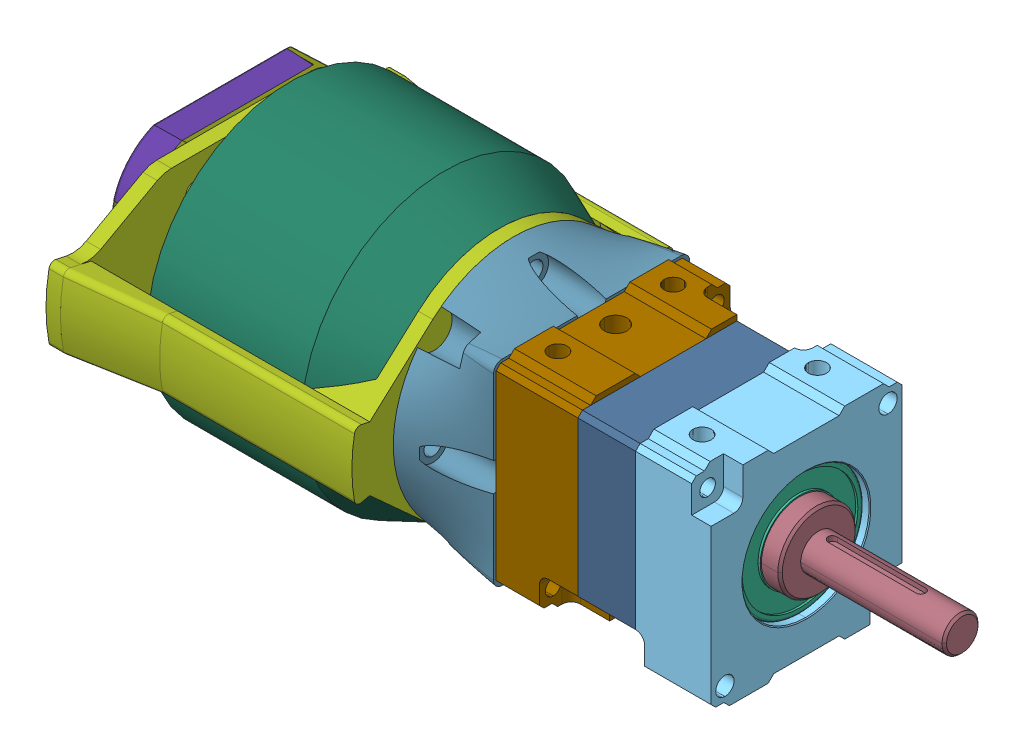
SolidWorks assembly Keda9to1, configuration Default. Lengths in mm.
Overall size (176.96 63 76.93).
46 component instances, 32 part files, 5 mates.
Components (placement in the parent):
- VersaPlanetary_v2_Single_Stage_10_1_with_BAG.STEP-1: VersaPlanetary_v2_Single_Stage_10_1_with_BAG.STEP [Default] at origin size (163.4 63.52 63.52)
  - 217-2820 Rev1_Public.STEP-1: 217-2820 Rev1_Public.STEP [Default] at (-4.6546 22.225 0) x (0 -0.456494 0.889726) z (-1 0 0) size (39.22 38.88 17.4)
    - 217-2625-100.STEP-1: 217-2625-100.STEP [Default] at origin size (39.22 38.88 12.7)
      - 217-2625-008 Rev1.STEP-1: 217-2625-008 Rev1.STEP [Default] at origin size (34.7 34.7 4.7)
      - 217-2625-010 Rev1.STEP-1: 217-2625-010 Rev1.STEP [Default] at (0 10.193 3.65) x (0.999813 0.019336 0) z (0 0 1) size (4 4 12)
      - 217-2625-010 Rev1.STEP-2: 217-2625-010 Rev1.STEP [Default] at (8.691 -5.3258 3.65) size (4 4 12)
      - 217-2625-010 Rev1.STEP-3: 217-2625-010 Rev1.STEP [Default] at (-8.691 -5.3258 3.65) size (4 4 12)
      - 217-2625-005 Rev1_Planet_Revolving_Follower01.STEP-1: 217-2625-005 Rev1_Planet_Revolving_Follower01.STEP [Default] at (8.691 -5.3258 6.35) x (0.932816 0.360354 0) z (0 0 1) size (16.89 16.89 8)
      - 217-2625-005 Rev1_Planet_Revolving_Follower01.STEP-2: 217-2625-005 Rev1_Planet_Revolving_Follower01.STEP [Default] at (-8.691 -5.3258 6.35) x (-0.932788 -0.360426 0) z (0 0 1) size (16.89 16.89 8)
      - 217-2625-005 Rev1_Planet_Revolving_Follower01.STEP-3: 217-2625-005 Rev1_Planet_Revolving_Follower01.STEP [Default] at (0 10.193 6.35) x (0.893583 0.448898 0) z (0 0 1) size (16.89 16.89 8)
    - 217-2625-007 Rev1_Public.STEP-1: 217-2625-007 Rev1_Public.STEP [Default] at (0 0 6.7) x (0.992772 0.120019 0) z (0 0 1) size (15.27 15.27 12.7)
  - 217-2625-026 Rev1.STEP-1: 217-2625-026 Rev1.STEP [Default] at (-6.5 22.225 0) x (0 -1 0) z (-1 0 0) size (44.45 42 18.12)
  - 217-2742-001 Rev4.STEP-1: 217-2742-001 Rev4.STEP [Default] at (0.2002 22.225 0) x (1 0 0) z (0 -0.092627 0.995701) size (7 28 28)
  - 217-2742-001 Rev4.STEP-2: 217-2742-001 Rev4.STEP [Default] at (8.2002 22.225 0) size (7 28 28)
  - 217-2625-017 Rev1_9714K61.STEP-1: 217-2625-017 Rev1_9714K61.STEP [Default] at (7.42 22.3002 -0.342) x (0 0.56703 0.823697) z (0 -0.823697 0.56703) size (28.51 4.98 27.43)
  - 217-2625-003 Rev1.STEP-1: 217-2625-003 Rev1.STEP [Default] at (7.4478 22.225 0) x (0 -1 0) z (1 0 0) size (17 17 64.11) (hidden)
  - 217-2625-018 Rev1_98541A410.STEP-1: 217-2625-018 Rev1_98541A410.STEP [Default] at (-0.7046 22.225 0) x (1 0 0) z (0 -0.017452 0.999848) size (1 19.6 17.4)
  - 832-1750-Ring-Gear-Screw_SSA0832-0500ZC.STEP-1: 832-1750-Ring-Gear-Screw_SSA0832-0500ZC.STEP [Default] at (-30.7 4.725 -17.5) x (0 0.997447 0.071411) z (0 -0.071411 0.997447) size (6.73 48.51 6.73) (hidden)
  - 832-1750-Ring-Gear-Screw_SSA0832-0500ZC.STEP-2: 832-1750-Ring-Gear-Screw_SSA0832-0500ZC.STEP [Default] at (-30.7 39.725 17.5) x (0 0.005929 0.999982) z (0 -0.999982 0.005929) size (6.73 48.51 6.73) (hidden)
  - 217-2625-025 Rev1.STEP-1: 217-2625-025 Rev1.STEP [Default] at (-23.2 22.225 0) x (0 -1 0) z (-1 0 0) size (44.45 42 18)
  - 217-4649-002 Rev1_SSA0832-0500ZC.STEP-1: 217-4649-002 Rev1_SSA0832-0500ZC.STEP [Default] at (-33.7 4.2645 17.9605) x (0 0.33842 -0.940995) z (0 0.940995 0.33842) size (6.73 16.76 6.73) (hidden)
  - 217-4649-002 Rev1_SSA0832-0500ZC.STEP-2: 217-4649-002 Rev1_SSA0832-0500ZC.STEP [Default] at (-33.7 40.1855 -17.9605) x (0 -0.308932 -0.951084) z (0 0.951084 -0.308932) size (6.73 16.76 6.73) (hidden)
  - 217-4649-006 Rev1_SSA0004-008BA.STEP-1: 217-4649-006 Rev1_SSA0004-008BA.STEP [Default] at (-30.7 22.225 12.5) x (0 0.5 -0.866025) z (0 -0.866025 -0.5) size (7 14 7) (hidden)
  - 217-4649-006 Rev1_SSA0004-008BA.STEP-2: 217-4649-006 Rev1_SSA0004-008BA.STEP [Default] at (-30.7 22.225 -12.5) x (0 -0.5 0.866025) z (0 0.866025 0.5) size (7 14 7) (hidden)
  - 217-2822-003 Rev4.STEP-1: 217-2822-003 Rev4.STEP [Default] at (-32.2 22.225 0) x (0 -1 0) z (-1 0 0) size (42 42 4.8) (hidden)
  - 217-3351 Rev2.STEP-1: 217-3351 Rev2.STEP [Default] at (-33.7 22.225 0) x (0 0 1) z (1 0 0) size (59.07 59.07 84.5) (hidden)
  - 217-2816-001 Rev1.STEP-1: 217-2816-001 Rev1.STEP [Default] at (-6.35 22.225 0) x (0 -1 0) z (1 0 0) size (42 42 14.51)
  - 217-4649-001 Rev1.STEP-1: 217-4649-001 Rev1.STEP [Default] at (-20.046 22.225 0) x (0 -1 0) z (1 0 0) size (18 18 13)
  - 217-4649-007 Rev1_94105A824.STEP-1: 217-4649-007 Rev1_94105A824.STEP [Default] at (-25.521 22.225 -6.7835) x (-0.996104 -0.088191 0) z (0 0 -1) size (4.83 4.83 4.77)
  - 217-2625-011 Rev1.STEP-1: 217-2625-011 Rev1.STEP [Default] at (-24.7818 22.225 0) x (0 0 1) z (0 -1 0) size (8.01 7.5 7.94) (hidden)
- VersaPlanetary_CIM_Motor_Output_Shaft_Kit_217-2893-1: VersaPlanetary_CIM_Motor_Output_Shaft_Kit_217-2893 [Default] at (7.4478 22.225 0) x (0 0 -1) z (1 0 0) size (17 17 57.85)
- KedaAdapter^Keda9to1-1: KedaAdapter^Keda9to1 [Default] at origin size (17.82 53.01 53.01) (virtual)
- 192kvMotorEncoded-1: 192kvMotorEncoded [Default] at (-51.0318 22.225 0) x (0 -1 0) z (0 0 -1) size (63 104.52 76.93)
  - BetterKEDA-1: BetterKEDA [Default] at origin size (63 104.52 63)
  - CUI_DEVICES_AMT102-0048-N2000-S-1: CUI_DEVICES_AMT102-0048-N2000-S [Default] at (0 65.12 0) x (1 0 0) z (0 1 0) size (36.33 46.21 9.2)
    - CUI_DEVICES_AMT102-0048-N2000-S.step-1: CUI_DEVICES_AMT102-0048-N2000-S.step [Default] at origin size (36.33 46.21 9.2)
      - AMT-102-Base-REV-K.step-1: AMT-102-Base-REV-K.step [Default] x (-1 0 0) z (0 0 -1) size (28.78 43.39 9.06)
      - AMT-102-Top-Cover-REV-H.step-1: AMT-102-Top-Cover-REV-H.step [Default] at (0 0 5.23) x (-1 0 0) z (0 0 -1) size (28.6 43.26 6.55)
      - AMT-Sleeve-REV-D_ 2 mm.step-1: AMT-Sleeve-REV-D_ 2 mm.step [Default] at (0 0 -2.42) x (0.999996 0.002864 0) z (0 0 1) size (10.79 10.79 7.8)
      - AMT-Hub-Top-REV-D1.step-1: AMT-Hub-Top-REV-D1.step [Default] at (0 0 2.13) x (0.999996 0.002864 0) z (0 0 1) size (14 14 5.67)
      - AMT-Hub-Bottom-REV-B.step-1: AMT-Hub-Bottom-REV-B.step [Default] at (0 0 2.43) x (0.999998 -0.001942 0) z (0 0 1) size (17.3 17.3 3.2)
      - AMT10X-Shaft-Adaptor-REV-E.step-1: AMT10X-Shaft-Adaptor-REV-E.step [Default] at (0 0 0.03) x (0.999996 0.002864 0) z (0 0 1) size (11.8 11.8 7.8)
      - Receiver-board.step-1: Receiver-board.step [Default] at (72.2834 -20.351 3.03) x (-1 0 0) z (0 0 -1) size (26.5 26.62 0.41)
      - Rotor-board-REV F.step-1: Rotor-board-REV F.step [Default] at (0 0 2.13) x (0.807874 -0.589355 0) z (0 0 1) size (26 26 0.3)
      - Transmitter-board AMT10_AMT-102.step-1: Transmitter-board AMT10_AMT-102.step [Default] at (19.1596 -17.1102 1.22) x (-1 0 0) z (0 0 -1) size (26.63 38.43 4.41)
  - Body^192kvMotorEncoded-1: Body^192kvMotorEncoded [Default] at origin size (53 64.53 76.93) (virtual)
Mates (geometry in assembly coordinates):
- Concentric2: concentric anti-aligned: cylinder of VersaPlanetary_v2_Single_Stage_10_1_with_BAG.STEP-1/217-2742-001 Rev4.STEP-2 through (8.2002 22.225 0) axis (-1 0 0) radius 7.5; cylinder of VersaPlanetary_CIM_Motor_Output_Shaft_Kit_217-2893-1 through (15.2002 22.225 0) axis (1 0 0) radius 8.5
- Coincident3: coincident anti-aligned: plane of VersaPlanetary_v2_Single_Stage_10_1_with_BAG.STEP-1/217-2742-001 Rev4.STEP-2 through (15.2002 29.725 0) normal (1 0 0); plane of VersaPlanetary_CIM_Motor_Output_Shaft_Kit_217-2893-1 through (15.2002 22.225 0) normal (-1 0 0)
- Concentric3: concentric aligned: cylinder of VersaPlanetary_v2_Single_Stage_10_1_with_BAG.STEP-1/217-4649-001 Rev1.STEP-1 through (-20.046 22.225 0) axis (-1 0 0) radius 4.005; cylinder of MotorEncoded-1/BetterKEDA-1 through (-21.5068 22.225 0) axis (-1 0 0) radius 4
- Coincident4: coincident anti-aligned: plane of KedaAdapter^Keda9to1-1 through (-51.0318 0 0) normal (-1 0 0); plane of MotorEncoded-1/BetterKEDA-1 through (-51.0318 22.225 0) normal (1 0 0)
- Coincident5: coincident anti-aligned: plane of 192kvMotorEncoded-1 through (-51.0318 22.225 0) normal (0 0 -1)
